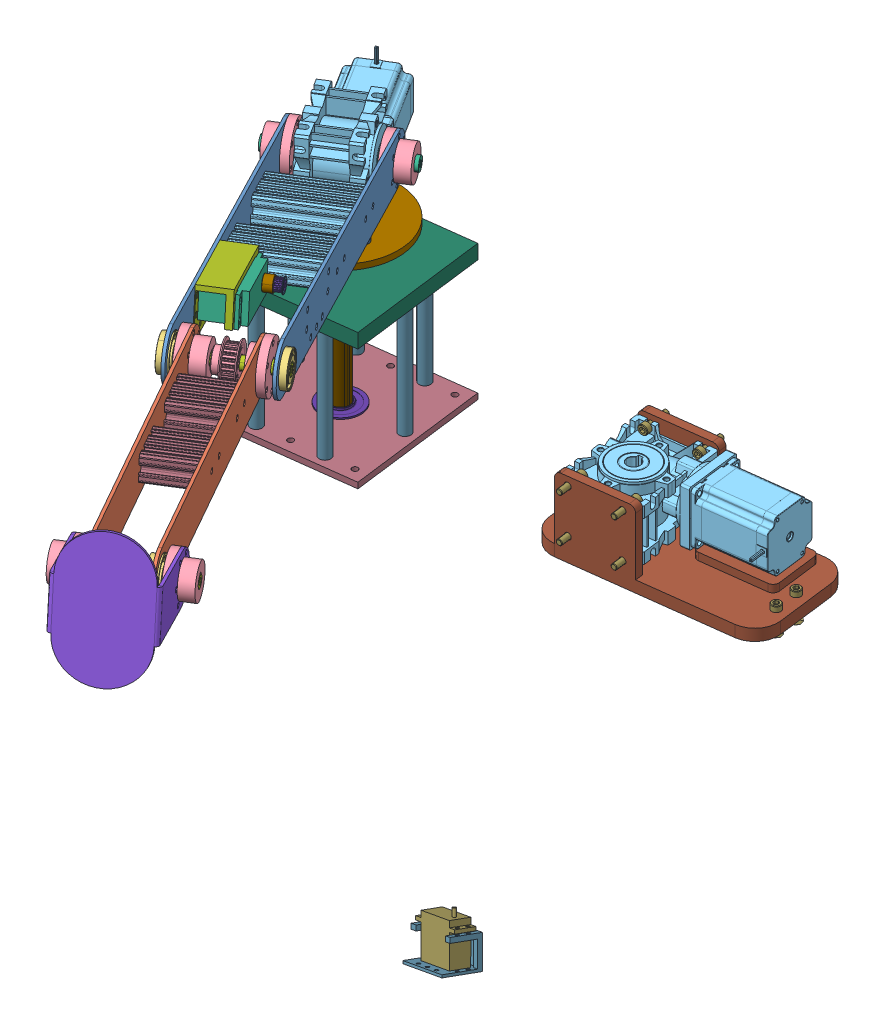
SolidWorks assembly Arm Assembly, configuration Default. Lengths in mm.
Overall size (689.03 483.25 867.03).
72 component instances, 32 part files, 136 mates.
Components (placement in the parent):
- Link 2-1: Link 2 [Default] at (-46.0857 347.5662 397.2138) x (0.521473 0.189246 0.832017) z (0.847329 0 -0.531069) size (457.2 50.8 3.17)
- Link 3-1: Link 3 [Default] at (228.0517 424.7546 698.466) x (0.527308 0.118805 0.841327) z (0.847329 0 -0.531069) size (406.4 50.8 3.17)
- Flanged Bearing-1: Flanged Bearing [Default] at (372.8529 441.7816 1027.9719) x (-0.531069 0 -0.847329) z (0.847329 0 -0.531069) size (38.1 38.1 12.7)
- Keyed hub-1: Keyed hub [Default] at (25.196 322.6251 358.2104) x (-0.50186 0.327073 -0.800725) z (-0.173699 -0.944999 -0.277139) size (50.8 25.4 50.8)
- Link 2-2: Link 2 [Default] at (29.3689 347.5662 349.9221) x (0.521473 0.189246 0.832017) z (0.847329 0 -0.531069) size (457.2 50.8 3.17)
- Link 3-2: Link 3 [Default] at (180.9848 424.7546 727.9655) x (0.527308 0.118805 0.841327) z (0.847329 0 -0.531069) size (406.4 50.8 3.17)
- Flanged Bearing-2: Flanged Bearing [Default] at (246.603 399.5345 690.4002) x (0.505623 0.305833 0.806729) z (0.847329 0 -0.531069) size (38.1 38.1 12.7)
- Flanged Bearing-3: Flanged Bearing [Default] at (417.1004 441.7816 1000.2394) x (0.490568 -0.383029 0.782708) z (-0.847329 0 0.531069) size (38.1 38.1 12.7)
- Keyed hub-2: Keyed hub [Default] at (175.8617 399.5345 734.7378) x (-0.425115 -0.599347 -0.678278) z (0.318295 -0.800489 0.507844) size (50.8 25.4 50.8)
- Keyed hub-3: Keyed hub [Default] at (-34.117 322.6251 395.3853) x (0.50186 -0.327073 0.800725) z (-0.173699 -0.944999 -0.277139) size (50.8 25.4 50.8)
- Keyed hub-4: Keyed hub [Default] at (239.0702 399.5345 695.1214) x (0.425115 0.599347 0.678278) z (0.318295 -0.800489 0.507844) size (50.8 25.4 50.8)
- Flanged Bearing-4: Flanged Bearing [Default] at (168.329 399.5345 739.459) x (-0.489048 0.389858 -0.780284) z (-0.847329 0 0.531069) size (38.1 38.1 12.7)
- Nema Stepper Motor-2: Nema Stepper Motor [Default] at (-44.1852 303.6559 313.4165) x (-0.531069 0 -0.847329) z (-0.847329 0 0.531069) size (171.01 100.01 63.01)
- Keyed Drive Shaft-1: Keyed Drive Shaft [Default] at (-114.1958 326.1952 444.2905) x (-0.50186 0.327073 -0.800725) z (0.847329 0 -0.531069) size (19.9 19.9 128.01)
- Keyed Shaft-1: Keyed Shaft [Default] at (155.1338 399.5345 747.7291) x (-0.425115 -0.599347 -0.678278) z (0.847329 0 -0.531069) size (12.7 12.5 104.14)
- Link 4-1: Link 4 [Default] at (433.2352 482.2587 1073.4043) x (0.847329 0 -0.531069) z (-0.10549 0.980073 -0.168311) size (90.37 102.6 133.86)
- Keyed hub-5: Keyed hub [Default] at (366.8892 441.7816 1031.7096) x (0.520486 0.198637 0.830444) z (0.10549 -0.980073 0.168311) size (50.8 25.4 50.8)
- Keyed hub-6: Keyed hub [Default] at (424.6331 441.7816 995.5182) x (-0.520486 -0.198637 -0.830444) z (0.10549 -0.980073 0.168311) size (50.8 25.4 50.8)
- Keyed Shaft-2: Keyed Shaft [Default] at (454.7641 441.7816 976.6334) x (0.520486 0.198637 0.830444) z (-0.847329 0 0.531069) size (12.7 12.5 104.14)
- Joint 2 Motor Plate-1: Joint 2 Motor Plate [Default] at (-4.244 255.2751 376.7854) x (0.215278 0 -0.976553) z (0.976553 0 0.215278) size (127 6.35 127)
- 4 mm M6 spacer-1: 4 mm M6 spacer [94669A162] at (1.753 263.6251 341.1619) x (-0.888418 0 -0.459036) z (0 -1 0) size (13 13 4)
- 4 mm M6 spacer-2: 4 mm M6 spacer [94669A162] at (30.4307 263.6251 386.9176) x (0.999963 0 0.008554) z (0 -1 0) size (13 13 4)
- 4 mm M6 spacer-3: 4 mm M6 spacer [94669A162] at (-38.9188 263.6251 366.6532) x (1 0 0) z (0 -1 0) size (13 13 4)
- 4 mm M6 spacer-4: 4 mm M6 spacer [94669A162] at (-10.2411 263.6251 412.409) x (1 0 0) z (0 -1 0) size (13 13 4)
- Motor Mount Joint 1 Assembly-1: Motor Mount Joint 1 Assembly [Default] at (255.7253 -1.2672 148.6448) x (0.992107 0 -0.125391) z (0.125391 0 0.992107) size (228.6 94.85 140.08)
  - Joint 1 Motor Holder Bracket-1: Joint 1 Motor Holder Bracket [Default] at (55.8829 79.1234 191.166) size (228.6 82.55 114.78)
  - Nema Stepper Motor-1: Nema Stepper Motor [Default] at (81.7887 128.4828 180.6968) x (1 0 0) z (0 1 0) size (171.01 100.01 63.01)
  - Flanged Bearing-1: Flanged Bearing [Default] at (6.9829 88.5722 199.666) x (0.99323 0 0.116162) z (0 -1 0) size (38.1 38.1 12.7)
  - socket head cap screw_am-7: socket head cap screw_am [B18.3.1M - 6 x 1.0 x 25 Hex SHCS -- 25NHX] at (-20.0631 152.4828 153.666) x (0 0 -1) z (0.990069 0.140585 0) size (31 10 10)
  - socket head cap screw_am-8: socket head cap screw_am [B18.3.1M - 6 x 1.0 x 25 Hex SHCS -- 25NHX] at (33.9369 152.4828 228.666) x (0 0 1) z (-1 0 0) size (31 10 10)
  - socket head cap screw_am-9: socket head cap screw_am [B18.3.1M - 6 x 1.0 x 25 Hex SHCS -- 25NHX] at (-20.0631 152.4828 228.666) x (0 0 1) z (0.381849 0.924225 0) size (31 10 10)
  - socket head cap screw_am-10: socket head cap screw_am [B18.3.1M - 6 x 1.0 x 25 Hex SHCS -- 25NHX] at (-20.0631 104.4828 153.666) x (0 0 -1) z (0.756248 0.654286 0) size (31 10 10)
  - socket head cap screw_am-11: socket head cap screw_am [B18.3.1M - 6 x 1.0 x 25 Hex SHCS -- 25NHX] at (33.9369 104.4828 150.5881) x (0 0 -1) z (0.923728 0.383049 0) size (31 10 10)
  - socket head cap screw_am-12: socket head cap screw_am [B18.3.1M - 6 x 1.0 x 25 Hex SHCS -- 25NHX] at (-45.7171 97.8234 212.366) x (0 -1 0) z (-0.546944 0 0.837169) size (31 10 10)
  - socket head cap screw_am-19: socket head cap screw_am [B18.3.1M - 6 x 1.0 x 25 Hex SHCS -- 25NHX] at (-45.7171 97.8234 186.966) x (0 -1 0) z (-0.546944 0 0.837169) size (31 10 10)
  - socket head cap screw_am-14: socket head cap screw_am [B18.3.1M - 6 x 1.0 x 25 Hex SHCS -- 25NHX] at (33.9369 152.4828 153.666) x (0 0 -1) z (0.923728 0.383049 0) size (31 10 10)
  - socket head cap screw_am-15: socket head cap screw_am [B18.3.1M - 6 x 1.0 x 25 Hex SHCS -- 25NHX] at (157.4829 97.8234 186.966) x (0 -1 0) z (-0.546944 0 0.837169) size (31 10 10)
  - socket head cap screw_am-16: socket head cap screw_am [B18.3.1M - 6 x 1.0 x 25 Hex SHCS -- 25NHX] at (-20.0631 104.4828 228.666) x (0 0 1) z (-1 0 0) size (31 10 10)
  - socket head cap screw_am-17: socket head cap screw_am [B18.3.1M - 6 x 1.0 x 25 Hex SHCS -- 25NHX] at (33.9369 104.4828 228.666) x (0 0 1) z (-1 0 0) size (31 10 10)
  - socket head cap screw_am-18: socket head cap screw_am [B18.3.1M - 6 x 1.0 x 25 Hex SHCS -- 25NHX] at (157.4829 97.8234 212.366) x (0 -1 0) z (-0.546944 0 0.837169) size (31 10 10)
- Joint 1 bottom plate-1: Joint 1 bottom plate [89155K113] at (-4.244 81.0311 376.7854) x (-0.125391 0 -0.992107) z (0.992107 0 -0.125391) size (152.4 6.35 152.4)
- Base post-1: Base post [8974K269] at (21.393 160.4061 309.54) x (-0.837169 0 -0.546944) z (0 -1 0) size (12.7 12.7 127)
- Base post-2: Base post [8974K269] at (-29.8811 160.4061 444.0308) x (-0.837169 0 -0.546944) z (0 -1 0) size (12.7 12.7 127)
- Base post-3: Base post [8974K269] at (37.3177 160.4061 435.5376) x (0.463623 0 0.886032) z (0 -1 0) size (12.7 12.7 127)
- Base post-4: Base post [8974K269] at (58.7548 160.4061 368.8231) x (-0.837169 0 -0.546944) z (0 -1 0) size (12.7 12.7 127)
- Base post-5: Base post [8974K269] at (-70.4278 160.4061 359.5483) x (-0.837169 0 -0.546944) z (0 -1 0) size (12.7 12.7 127)
- Base post-6: Base post [8974K269] at (-45.8058 160.4061 318.0332) x (-0.837169 0 -0.546944) z (0 -1 0) size (12.7 12.7 127)
- Base post-7: Base post [8974K269] at (-64.0579 160.4061 409.9473) x (-0.837169 0 -0.546944) z (0 -1 0) size (12.7 12.7 127)
- Joint 1 top plate-1: Joint 1 top plate [89155K143] at (-4.244 219.1436 376.7854) x (-0.125391 0 -0.992107) z (0.992107 0 -0.125391) size (152.4 15.88 152.4)
- Tapered-Roller Bearing-1: Tapered-Roller Bearing [5709K77] at (-4.244 223.5886 376.7854) x (1 0 0) z (0 -1 0) size (45.24 45.24 17.1)
- base Ball Bearing 0.75 in-1: base Ball Bearing 0.75 in [6384K367] at (-4.244 79.4436 376.7854) x (1 0 0) z (0 -1 0) size (44.45 44.45 14.27)
- keyed shaft 0.75 in bore 9 in-1: keyed shaft 0.75 in bore 9 in [Default] at (-4.244 155.2626 376.7854) x (0.215278 0 -0.976553) z (0 -1 0) size (19.05 18.75 228.6)
- 0.75 in shaft hub-1: 0.75 in shaft hub [Default] at (-4.244 248.9251 376.7854) x (-0.215278 0 0.976553) z (0 -1 0) size (63.5 63.5 19.49)
- Clamping Two-Piece Shaft Collar 0.75 in-1: Clamping Two-Piece Shaft Collar 0.75 in [6436K16] at (-4.244 240.9876 376.7854) x (0.996685 0 0.081358) z (0 1 0) size (38.06 38.1 12.77)
- T-slot Slider-1: T-slot Slider [5278N52] at (236.9979 67.7205 365.0672) x (-0.837169 0 -0.546944) z (0 1 0) size (10 9.8 4.82)
- T-slot Slider-2: T-slot Slider [5278N52] at (233.8129 65.4156 339.8677) x (-0.837169 0 -0.546944) z (0 1 0) size (10 9.8 4.82)
- T-slot Slider-3: T-slot Slider [5278N52] at (438.5941 68.7454 339.5877) x (-0.838988 0 -0.544149) z (0 1 0) size (10 9.8 4.82)
- T-slot Slider-4: T-slot Slider [5278N52] at (435.4091 66.889 314.3882) x (-0.837169 0 -0.546944) z (0 1 0) size (10 9.8 4.82)
- joint3pulley-1: joint3pulley [6495K752] at (208.3994 399.5345 714.3446) x (-0.496066 -0.357037 -0.791481) z (-0.847329 0 0.531069) size (38.1 38.1 22.23)
- 8020tframeforjoint3-1: 8020tframeforjoint3 [47065T653] at (20.3369 341.8525 478.9955) x (-0.100502 0.98193 -0.160353) z (0.847329 0 -0.531069) size (25.4 50.8 85.85)
- 8020tframeforjoint3-2: 8020tframeforjoint3 [47065T653] at (73.3185 361.0798 563.5284) x (-0.100502 0.98193 -0.160353) z (0.847329 0 -0.531069) size (25.4 50.8 85.85)
- 80 kg-1: 80 kg [Default] at (126.7022 373.3731 665.4861) x (-0.521473 -0.189246 -0.832017) z (0.100502 -0.98193 0.160353) size (82 48 30)
- servobracket_80kg-1: servobracket_80kg [Default] at (108.1358 376.7277 637.298) x (-0.521473 -0.189246 -0.832017) z (0.100502 -0.98193 0.160353) size (87.12 31.24 59.67)
- 3422-0004-0020 assembly.STEP-1: 3422-0004-0020 assembly.STEP [Default] at (106.5575 368.2135 573.9097) x (-0.472745 -0.455616 -0.754272) z (0.241963 -0.890177 0.386056) size (15 18 15.01)
  - 3422-0004-0020 core.STEP-1: 3422-0004-0020 core.STEP [Default] at (-35.1952 21.4358 6.7264) size (12.22 18 12.22)
  - 3422 series barrel.STEP-1: 3422 series barrel.STEP [Default] at (-35.1952 8.9358 6.7264) x (1 0 0) z (0 1 0) size (15 15.01 9)
  - 3422 series flange.STEP-1: 3422 series flange.STEP [Default] at (-35.1952 24.9358 6.7264) x (1 0 0) z (0 1 0) size (15 15 1)
  - 2806-0005-0005_91390A117.STEP-1: 2806-0005-0005_91390A117.STEP [Default] at (-35.1952 13.4358 11.638) x (-0.412538 -0.91094 0) z (0 0 1) size (5.01 5.01 5.01)
- 25 kg-1: 25 kg [Default] at (537.5356 49.5478 829.9464) x (0.939938 0.302082 0.158944) z (-0.225843 0.201201 0.953159) size (55 48 20)
- 8020tframeforjoint4-1: 8020tframeforjoint4 [47065T653] at (290.0659 408.5875 752.4523) x (-0.063094 0.992918 -0.100667) z (-0.847329 0 0.531069) size (25.4 50.8 52.32)
- 8020tframeforjoint4-2: 8020tframeforjoint4 [47065T653] at (336.9436 419.1492 827.2463) x (0.063094 -0.992918 0.100667) z (-0.847329 0 0.531069) size (25.4 50.8 52.32)
- 25kgservobracket2-3: 25kgservobracket2 [Default] at (940.3101 476.6609 1737.7737) x (-0.939938 -0.302082 -0.158944) z (-0.255952 0.931807 -0.25734) size (55.12 37.85 31.5)
Mates (geometry in assembly coordinates):
- Concentric3: concentric aligned: cylinder of Keyed hub-1 through (31.9217 322.6251 353.9951) axis (0.847329 0 -0.531069) radius 17.4625; cylinder of Link 2-2 through (31.9217 322.6251 353.9951) axis (0.847329 0 -0.531069) radius 17.4625
- Coincident2: coincident anti-aligned: plane of Keyed hub-1 through (31.9217 322.6251 353.9951) normal (0.847329 0 -0.531069); plane of Link 2-2 through (31.9217 322.6251 353.9951) normal (-0.847329 0 0.531069)
- Concentric4: concentric aligned: cylinder of Keyed hub-1 through (21.3415 329.5205 337.1142) axis (0.847329 0 -0.531069) radius 2.5527; cylinder of Link 2-2 through (24.0317 329.5205 335.4281) axis (0.847329 0 -0.531069) radius 2.5527
- Concentric5: concentric anti-aligned: cylinder of Link 2-1 through (-43.5329 322.6251 401.2868) axis (0.847329 0 -0.531069) radius 17.4625; cylinder of Keyed hub-3 through (-40.8427 322.6251 399.6006) axis (-0.847329 0 0.531069) radius 17.4625
- Coincident3: coincident anti-aligned: plane of Link 2-1 through (-40.8427 322.6251 399.6006) normal (0.847329 0 -0.531069); plane of Keyed hub-3 through (-40.8427 322.6251 399.6006) normal (-0.847329 0 0.531069)
- Concentric7: concentric anti-aligned: cylinder of Link 2-1 through (-38.7239 301.9241 402.9812) axis (0.847329 0 -0.531069) radius 2.5527; cylinder of Keyed hub-3 through (-38.7239 301.9241 402.9812) axis (-0.847329 0 0.531069) radius 2.5527
- Concentric8: concentric anti-aligned: cylinder of Keyed hub-1 through (25.196 322.6251 358.2104) axis (0.847329 0 -0.531069) radius 6.35; cylinder of Keyed hub-3 through (-34.117 322.6251 395.3853) axis (-0.847329 0 0.531069) radius 6.35
- Coincident5: coincident aligned: plane of Keyed hub-1 through (25.9927 322.1059 359.4816) normal (-0.50186 0.327073 -0.800725); plane of Keyed hub-3 through (-33.3203 322.1059 396.6564) normal (-0.50186 0.327073 -0.800725)
- Concentric9: concentric aligned: cylinder of Link 2-2 through (243.8481 399.5345 692.1268) axis (0.847329 0 -0.531069) radius 17.4625; cylinder of Flanged Bearing-2 through (251.9835 399.5345 687.0279) axis (0.847329 0 -0.531069) radius 17.4625
- Concentric10: concentric anti-aligned: cylinder of Link 2-1 through (168.3935 399.5345 739.4185) axis (0.847329 0 -0.531069) radius 17.4625; cylinder of Flanged Bearing-4 through (162.9484 399.5345 742.8313) axis (-0.847329 0 0.531069) radius 17.4625
- Concentric11: concentric anti-aligned: cylinder of Link 3-1 through (229.6543 399.5345 701.0229) axis (0.847329 0 -0.531069) radius 17.4625; cylinder of Keyed hub-4 through (232.3445 399.5345 699.3368) axis (-0.847329 0 0.531069) radius 17.4625
- Coincident8: coincident anti-aligned: plane of Link 3-1 through (232.3445 399.5345 699.3368) normal (0.847329 0 -0.531069); plane of Keyed hub-4 through (232.3445 399.5345 699.3368) normal (-0.847329 0 0.531069)
- Concentric12: concentric anti-aligned: cylinder of Link 3-1 through (231.0144 420.4672 697.2145) axis (0.847329 0 -0.531069) radius 2.5527; cylinder of Keyed hub-4 through (231.0144 420.4672 697.2145) axis (-0.847329 0 0.531069) radius 2.5527
- Concentric13: concentric aligned: cylinder of Link 3-2 through (182.5874 399.5345 730.5225) axis (0.847329 0 -0.531069) radius 17.4625; cylinder of Keyed hub-2 through (182.5874 399.5345 730.5225) axis (0.847329 0 -0.531069) radius 17.4625
- Coincident9: coincident anti-aligned: plane of Link 3-2 through (182.5874 399.5345 730.5225) normal (-0.847329 0 0.531069); plane of Keyed hub-2 through (182.5874 399.5345 730.5225) normal (0.847329 0 -0.531069)
- Concentric14: concentric aligned: cylinder of Link 3-2 through (183.9475 420.4672 726.714) axis (0.847329 0 -0.531069) radius 2.5527; cylinder of Keyed hub-2 through (181.2572 420.4672 728.4002) axis (0.847329 0 -0.531069) radius 2.5527
- Concentric15: concentric anti-aligned: cylinder of Keyed hub-2 through (175.8617 399.5345 734.7378) axis (0.847329 0 -0.531069) radius 6.35; cylinder of Keyed hub-4 through (239.0702 399.5345 695.1214) axis (-0.847329 0 0.531069) radius 6.35
- Coincident10: coincident aligned: plane of Keyed hub-2 through (175.1868 398.5831 733.661) normal (0.425115 0.599347 0.678278); plane of Keyed hub-4 through (238.3953 398.5831 694.0447) normal (0.425115 0.599347 0.678278)
- Concentric16: concentric aligned: cylinder of Flanged Bearing-2 through (251.9835 399.5345 687.0279) axis (0.847329 0 -0.531069) radius 6.35; cylinder of Keyed hub-2 through (175.8617 399.5345 734.7378) axis (0.847329 0 -0.531069) radius 6.35
- Concentric17: concentric aligned: cylinder of Flanged Bearing-1 through (378.2334 441.7816 1024.5996) axis (0.847329 0 -0.531069) radius 17.4625; cylinder of Link 3-2 through (370.098 441.7816 1029.6985) axis (0.847329 0 -0.531069) radius 17.4625
- Coincident13: coincident anti-aligned: plane of Flanged Bearing-1 through (370.098 459.2441 1029.6985) normal (0.847329 0 -0.531069); plane of Link 3-2 through (182.5874 399.5345 730.5225) normal (-0.847329 0 0.531069)
- Concentric18: concentric anti-aligned: cylinder of Link 3-1 through (417.1649 441.7816 1000.199) axis (0.847329 0 -0.531069) radius 17.4625; cylinder of Flanged Bearing-3 through (411.7198 441.7816 1003.6117) axis (-0.847329 0 0.531069) radius 17.4625
- Coincident14: coincident anti-aligned: plane of Link 3-1 through (232.3445 399.5345 699.3368) normal (0.847329 0 -0.531069); plane of Flanged Bearing-3 through (423.4073 457.9123 1004.1803) normal (-0.847329 0 0.531069)
- Concentric21: concentric anti-aligned: cylinder of Keyed hub-1 through (25.196 322.6251 358.2104) axis (0.847329 0 -0.531069) radius 6.35; cylinder of Keyed Drive Shaft-1 through (49.7685 322.6251 342.8094) axis (-0.847329 0 0.531069) radius 7
- Parallel1: parallel anti-aligned: plane of Keyed hub-1 through (25.9927 322.1059 359.4816) normal (-0.50186 0.327073 -0.800725); plane of Keyed Drive Shaft-1 through (-2.2852 326.816 380.2685) normal (0.50186 -0.327073 0.800725)
- Coincident18: coincident anti-aligned: plane of Keyed hub-3 through (-34.117 322.6251 395.3853) normal (0.847329 0 -0.531069); plane of Keyed Drive Shaft-1 through (-32.3521 328.5578 398.2011) normal (-0.847329 0 0.531069)
- Coincident19: coincident anti-aligned: plane of Keyed hub-1 through (25.196 322.6251 358.2104) normal (-0.847329 0 0.531069); plane of Keyed Drive Shaft-1 through (26.9609 328.5578 361.0263) normal (0.847329 0 -0.531069)
- Concentric22: concentric anti-aligned: cylinder of Keyed hub-2 through (175.8617 399.5345 734.7378) axis (0.847329 0 -0.531069) radius 6.35; cylinder of Keyed Shaft-1 through (251.9835 399.5345 687.0279) axis (-0.847329 0 0.531069) radius 6.35
- Coincident20: coincident aligned: plane of Keyed hub-2 through (175.1868 398.5831 733.661) normal (0.425115 0.599347 0.678278); plane of Keyed Shaft-1 through (249.7968 402.3852 683.539) normal (0.425115 0.599347 0.678278)
- Coincident22: coincident anti-aligned: plane of Link 2-1 through (-40.8427 322.6251 399.6006) normal (0.847329 0 -0.531069); plane of Flanged Bearing-4 through (167.4683 383.4537 731.9639) normal (-0.847329 0 0.531069)
- Distance1: distance = 2.54 mm anti-aligned: plane of Flanged Bearing-4 through (171.3272 388.9387 732.2858) normal (0.847329 0 -0.531069); plane of Keyed hub-2 through (175.8617 399.5345 734.7378) normal (-0.847329 0 0.531069)
- Coincident24: coincident anti-aligned: plane of Link 2-2 through (31.9217 322.6251 353.9951) normal (-0.847329 0 0.531069); plane of Flanged Bearing-2 through (246.6844 382.9087 696.6521) normal (0.847329 0 -0.531069)
- Distance2: distance = 2.54 mm anti-aligned: plane of Keyed hub-4 through (239.0702 399.5345 695.1214) normal (0.847329 0 -0.531069); plane of Flanged Bearing-2 through (243.0912 388.5796 696.7542) normal (-0.847329 0 0.531069)
- Coincident26: coincident aligned: plane of Flanged Bearing-2 through (253.0149 393.4888 688.6735) normal (0.847329 0 -0.531069); plane of Keyed Shaft-1 through (251.9835 399.5345 687.0279) normal (0.847329 0 -0.531069)
- Concentric23: concentric anti-aligned: cylinder of Link 4-1 through (434.0491 441.7816 989.6167) axis (-0.847329 0 0.531069) radius 17.4625; cylinder of Keyed hub-6 through (431.3588 441.7816 991.3029) axis (0.847329 0 -0.531069) radius 17.4625
- Concentric24: concentric anti-aligned: cylinder of Link 4-1 through (423.9463 457.5815 979.4762) axis (-0.847329 0 0.531069) radius 2.5527; cylinder of Keyed hub-6 through (423.9463 457.5815 979.4762) axis (0.847329 0 -0.531069) radius 2.5527
- Coincident27: coincident anti-aligned: plane of Link 4-1 through (490.1801 490.4056 1085.1531) normal (-0.847329 0 0.531069); plane of Keyed hub-6 through (431.3588 441.7816 991.3029) normal (0.847329 0 -0.531069)
- Concentric25: concentric anti-aligned: cylinder of Link 4-1 through (357.4733 441.7816 1037.6111) axis (0.847329 0 -0.531069) radius 17.4625; cylinder of Keyed hub-5 through (360.1635 441.7816 1035.925) axis (-0.847329 0 0.531069) radius 17.4625
- Concentric26: concentric anti-aligned: cylinder of Link 4-1 through (352.7511 457.5815 1024.0983) axis (0.847329 0 -0.531069) radius 2.5527; cylinder of Keyed hub-5 through (352.7511 457.5815 1024.0983) axis (-0.847329 0 0.531069) radius 2.5527
- Concentric27: concentric anti-aligned: cylinder of Keyed hub-5 through (366.8892 441.7816 1031.7096) axis (-0.847329 0 0.531069) radius 6.35; cylinder of Keyed Shaft-2 through (357.9145 441.7816 1037.3346) axis (0.847329 0 -0.531069) radius 6.35
- Coincident31: coincident aligned: plane of Keyed hub-5 through (366.0629 441.4662 1030.3913) normal (0.520486 0.198637 0.830444); plane of Keyed Shaft-2 through (356.5871 446.1214 1035.2168) normal (0.520486 0.198637 0.830444)
- Coincident32: coincident aligned: plane of Keyed hub-6 through (446.1553 441.7816 982.0291) normal (0.847329 0 -0.531069); plane of Keyed Shaft-2 through (446.1553 441.7816 982.0291) normal (0.847329 0 -0.531069)
- Coincident34: coincident anti-aligned: plane of Link 4-1 through (418.9848 490.4056 1129.7752) normal (0.847329 0 -0.531069); plane of Keyed hub-5 through (360.1635 441.7816 1035.925) normal (-0.847329 0 0.531069)
- Coincident36: coincident aligned: plane of Keyed hub-6 through (425.4594 442.0969 996.8366) normal (-0.520486 -0.198637 -0.830444); plane of Keyed Shaft-2 through (358.2397 446.7521 1037.8535) normal (-0.520486 -0.198637 -0.830444)
- Concentric28: concentric anti-aligned: cone of Flanged Bearing-3 through (421.9135 441.7816 997.2228) axis (-0.847329 0 0.531069); cylinder of Keyed Shaft-2 through (357.9145 441.7816 1037.3346) axis (0.847329 0 -0.531069) radius 6.35
- Distance3: distance = 2.54 mm anti-aligned: plane of Flanged Bearing-3 through (424.8214 452.4103 1000.6015) normal (0.847329 0 -0.531069); plane of Keyed hub-6 through (424.6331 441.7816 995.5182) normal (-0.847329 0 0.531069)
- Coincident38: coincident anti-aligned: plane of Top base plate-1 through (74.0847 244.0001 261.2257) normal (0 -1 0); plane of arm base spacer small part-1 through (130.8381 244.0001 364.6329) normal (0 1 0)
- Coincident40: coincident anti-aligned: plane of Top base plate-1 through (74.0847 244.0001 261.2257) normal (0 -1 0); plane of arm base spacer large part-1 through (32.1724 244.0001 346.1862) normal (0 1 0)
- Coincident45: coincident anti-aligned: plane of Bearing other part-1 through (32.1724 247.1751 346.1862) normal (0 -1 0); plane of Top base plate-1 through (74.0847 247.1751 261.2257) normal (0 1 0)
- Concentric32: concentric aligned: cylinder of Bearing other part-1 through (32.1724 257.1751 346.1862) axis (0 -1 0) radius 70; circle of arm base spacer large part-1
- Coincident57: coincident aligned: plane of Top base plate-1 through (-6.0476 247.1751 446.2586) normal (0.059501 0 0.998228); plane of arm base spacer large part-1 through (84.7912 244.0001 440.844) normal (0.059501 0 0.998228)
- Coincident58: coincident aligned: plane of Top base plate-1 through (-75.7951 247.1751 376.9496) normal (-0.998228 0 0.059501); plane of arm base spacer large part-1 through (-75.8042 244.0001 376.7975) normal (-0.998228 0 0.059501)
- Concentric37: concentric aligned: cylinder of Top base plate-1 through (130.8381 247.1751 364.6329) axis (0 -1 0) radius 15; cylinder of arm base spacer small part-1 through (130.8381 244.0001 364.6329) axis (0 -1 0) radius 15
- Coincident59: coincident aligned: plane of Top base plate-1 through (145.8116 247.1751 363.7404) normal (0.998228 0 -0.059501); plane of arm base spacer small part-1 through (145.8116 244.0001 363.7404) normal (0.998228 0 -0.059501)
- Parallel2: parallel aligned: plane of Nema Stepper Motor-3 through (350.3499 203.0272 320.7095) normal (0 1 0); plane of Top base plate-1 through (74.0847 247.1751 261.2257) normal (0 1 0)
- Parallel3: parallel anti-aligned: plane of Nema Stepper Motor-3 through (312.2058 175.0272 353.0364) normal (-0.998228 0 0.059501); plane of arm base spacer small part-1 through (145.8116 244.0001 363.7404) normal (0.998228 0 -0.059501)
- Coincident61: coincident anti-aligned: plane of Nema Stepper Motor-2 through (-1.9757 265.6251 328.0385) normal (0 -1 0); plane of 4 mm M6 spacer-1 through (1.753 265.6251 341.1619) normal (0 1 0)
- Concentric43: concentric aligned: cylinder of Keyed hub-1 through (31.9217 322.6251 353.9951) axis (0.847329 0 -0.531069) radius 17.4625; cylinder of Nema Stepper Motor-2 through (-83.0293 322.6251 426.0414) axis (0.847329 0 -0.531069) radius 7
- Coincident65: coincident anti-aligned: plane of Nema Stepper Motor-2 through (22.2327 322.6251 360.0729) normal (0.847329 0 -0.531069); plane of Keyed Drive Shaft-1 through (22.2304 322.6251 360.0692) normal (-0.847329 0 0.531069)
- Concentric44: concentric aligned: cylinder of Joint 1 bottom plate-1 through (58.7548 83.9521 368.8231) axis (0 1 0) radius 1.905; cylinder of Base post-4 through (58.7548 84.2061 368.8231) axis (0 1 0) radius 6.35
- Concentric45: concentric aligned: cylinder of Joint 1 bottom plate-1 through (37.3177 83.9521 435.5376) axis (0 1 0) radius 1.905; cylinder of Base post-3 through (37.3177 84.2061 435.5376) axis (0 1 0) radius 6.35
- Concentric46: concentric aligned: cylinder of Joint 1 bottom plate-1 through (-29.8811 83.9521 444.0308) axis (0 1 0) radius 1.905; cylinder of Base post-2 through (-29.8811 84.2061 444.0308) axis (0 1 0) radius 6.35
- Concentric47: concentric aligned: cylinder of Joint 1 bottom plate-1 through (21.393 83.9521 309.54) axis (0 1 0) radius 1.905; cylinder of Base post-1 through (21.393 84.2061 309.54) axis (0 1 0) radius 6.35
- Concentric48: concentric aligned: cylinder of Joint 1 bottom plate-1 through (-45.8058 83.9521 318.0332) axis (0 1 0) radius 1.905; cylinder of Base post-6 through (-45.8058 84.2061 318.0332) axis (0 1 0) radius 6.35
- Concentric49: concentric aligned: cylinder of Joint 1 bottom plate-1 through (-64.0579 83.9521 409.9473) axis (0 1 0) radius 1.905; cylinder of Base post-7 through (-64.0579 84.2061 409.9473) axis (0 1 0) radius 6.35
- Concentric50: concentric aligned: cylinder of Joint 1 bottom plate-1 through (-70.4278 83.9521 359.5483) axis (0 1 0) radius 1.905; cylinder of Base post-5 through (-70.4278 84.2061 359.5483) axis (0 1 0) radius 6.35
- Coincident66: coincident anti-aligned: plane of Joint 1 bottom plate-1 through (80.9094 84.2061 442.8292) normal (0 1 0); plane of Base post-4 through (58.7548 84.2061 368.8231) normal (0 -1 0)
- Coincident67: coincident anti-aligned: plane of Joint 1 bottom plate-1 through (80.9094 84.2061 442.8292) normal (0 1 0); plane of Base post-3 through (37.3177 84.2061 435.5376) normal (0 -1 0)
- Coincident68: coincident anti-aligned: plane of Joint 1 bottom plate-1 through (80.9094 84.2061 442.8292) normal (0 1 0); plane of Base post-2 through (-29.8811 84.2061 444.0308) normal (0 -1 0)
- Coincident69: coincident anti-aligned: plane of Joint 1 bottom plate-1 through (80.9094 84.2061 442.8292) normal (0 1 0); plane of Base post-7 through (-64.0579 84.2061 409.9473) normal (0 -1 0)
- Coincident70: coincident anti-aligned: plane of Joint 1 bottom plate-1 through (80.9094 84.2061 442.8292) normal (0 1 0); plane of Base post-1 through (21.393 84.2061 309.54) normal (0 -1 0)
- Coincident71: coincident anti-aligned: plane of Joint 1 bottom plate-1 through (80.9094 84.2061 442.8292) normal (0 1 0); plane of Base post-6 through (-45.8058 84.2061 318.0332) normal (0 -1 0)
- Coincident72: coincident anti-aligned: plane of Joint 1 bottom plate-1 through (80.9094 84.2061 442.8292) normal (0 1 0); plane of Base post-5 through (-70.4278 84.2061 359.5483) normal (0 -1 0)
- Coincident73: coincident aligned: plane of Joint 1 bottom plate-1 through (71.3545 81.0311 367.2306) normal (0.992107 0 -0.125391); plane of Joint 1 top plate-1 through (71.3545 219.1436 367.2306) normal (0.992107 0 -0.125391)
- Coincident74: coincident aligned: plane of Joint 1 bottom plate-1 through (80.9094 77.8561 442.8292) normal (0.125391 0 0.992107); plane of Joint 1 top plate-1 through (80.9094 211.2061 442.8292) normal (0.125391 0 0.992107)
- Coincident75: coincident anti-aligned: plane of Base post-3 through (37.3177 211.2061 435.5376) normal (0 1 0); plane of Joint 1 top plate-1 through (61.7997 211.2061 291.632) normal (0 -1 0)
- Parallel5: parallel aligned: plane of Motor Mount Joint 1 Assembly-1/Joint 1 Motor Holder Bracket-1 through (228.936 90.5561 402.5641) normal (0.125391 0 0.992107); plane of Joint 1 bottom plate-1 through (80.9094 77.8561 442.8292) normal (0.125391 0 0.992107)
- Coincident79: coincident anti-aligned: plane of Joint 1 top plate-1 through (-4.244 217.5561 376.7854) normal (0 1 0); plane of Tapered-Roller Bearing-1 through (-4.244 217.5561 399.4073) normal (0 -1 0)
- Concentric51: concentric anti-aligned: cylinder of Joint 1 top plate-1 through (-4.244 217.5561 376.7854) axis (0 1 0) radius 22.6219; cylinder of Tapered-Roller Bearing-1 through (-4.244 223.5886 376.7854) axis (0 -1 0) radius 22.6219
- Coincident80: coincident anti-aligned: plane of Nema Stepper Motor-2 through (-1.9757 265.6251 328.0385) normal (0 -1 0); plane of 4 mm M6 spacer-2 through (30.4307 265.6251 386.9176) normal (0 1 0)
- Coincident81: coincident anti-aligned: plane of Nema Stepper Motor-2 through (-1.9757 265.6251 328.0385) normal (0 -1 0); plane of 4 mm M6 spacer-4 through (-10.2411 265.6251 412.409) normal (0 1 0)
- Concentric52: concentric anti-aligned: cylinder of Joint 1 bottom plate-1 through (-4.244 77.8561 376.7854) axis (0 1 0) radius 20.6375; cylinder of base Ball Bearing 0.75 in-1 through (-4.244 73.0936 376.7854) axis (0 -1 0) radius 20.6375
- Coincident82: coincident anti-aligned: plane of Joint 1 bottom plate-1 through (80.9094 84.2061 442.8292) normal (0 1 0); plane of base Ball Bearing 0.75 in-1 through (-4.244 84.2061 395.7927) normal (0 -1 0)
- Concentric53: concentric anti-aligned: cylinder of base Ball Bearing 0.75 in-1 through (-4.244 73.0936 376.7854) axis (0 -1 0) radius 9.525; cylinder of keyed shaft 0.75 in bore-1 through (-4.244 -126.3486 376.7854) axis (0 1 0) radius 9.525
- Concentric54: concentric anti-aligned: cylinder of base Ball Bearing 0.75 in-1 through (-4.244 73.0936 376.7854) axis (0 -1 0) radius 9.525; cylinder of keyed shaft 0.75 in bore 9 in-1 through (-4.244 40.9626 376.7854) axis (0 1 0) radius 9.525
- Coincident83: coincident aligned: plane of Motor Mount Joint 1 Assembly-1/Joint 1 Motor Holder Bracket-1 through (335.1377 77.8561 331.2948) normal (0 -1 0); plane of Joint 1 bottom plate-1 through (61.7997 77.8561 291.632) normal (0 -1 0)
- Concentric55: concentric aligned: cylinder of Joint 2 Motor Plate-1 through (-4.244 255.2751 376.7854) axis (0 1 0) radius 20.6375; circle of 0.75 in shaft hub-1
- Concentric56: concentric anti-aligned: cylinder of Joint 2 Motor Plate-1 through (-25.6499 255.2751 390.4583) axis (0 1 0) radius 3.175; circle of 0.75 in shaft hub-1
- Concentric57: concentric aligned: cylinder of keyed shaft 0.75 in bore 9 in-1 through (-4.244 40.9626 376.7854) axis (0 1 0) radius 9.525; cylinder of 0.75 in shaft hub-1 through (-4.244 247.3376 376.7854) axis (0 1 0) radius 9.525
- Parallel6: parallel aligned: plane of keyed shaft 0.75 in bore 9 in-1 through (2.212 40.9626 380.6536) normal (0.215278 0 -0.976553); plane of 0.75 in shaft hub-1 through (6.8704 248.9251 381.674) normal (0.215278 0 -0.976553)
- Coincident90: coincident anti-aligned: plane of Joint 2 Motor Plate-1 through (-4.244 255.2751 376.7854) normal (0 -1 0); plane of 0.75 in shaft hub-1 through (-4.244 255.2751 376.7854) normal (0 1 0)
- Concentric60: concentric anti-aligned: cylinder of keyed shaft 0.75 in bore 9 in-1 through (-4.244 40.9626 376.7854) axis (0 1 0) radius 9.525; cylinder of Clamping Two-Piece Shaft Collar 0.75 in-1 through (-4.244 247.3376 376.7854) axis (0 -1 0) radius 9.525
- Distance7: distance = 1.5875 mm anti-aligned: plane of Tapered-Roller Bearing-1 through (-4.244 233.0501 386.3104) normal (0 1 0); plane of Clamping Two-Piece Shaft Collar 0.75 in-1 through (-4.244 234.6376 376.7854) normal (0 -1 0)
- Distance8: distance = 1.5875 mm anti-aligned: plane of Clamping Two-Piece Shaft Collar 0.75 in-1 through (-4.244 247.3376 376.7854) normal (0 1 0); plane of 0.75 in shaft hub-1 through (-4.244 248.9251 376.7854) normal (0 -1 0)
- Distance9: distance = 1.5875 mm aligned: plane of keyed shaft 0.75 in bore 9 in-1 through (-4.244 269.5626 376.7854) normal (0 1 0); plane of 0.75 in shaft hub-1 through (-4.244 267.9751 376.7854) normal (0 1 0)
- Coincident95: coincident anti-aligned: plane of Nema Stepper Motor-2 through (-1.9757 265.6251 328.0385) normal (0 -1 0); plane of 4 mm M6 spacer-3 through (-38.9188 265.6251 366.6532) normal (0 1 0)
- Coincident96: coincident anti-aligned: plane of Joint 2 Motor Plate-1 through (-4.244 261.6251 376.7854) normal (0 1 0); plane of 4 mm M6 spacer-3 through (-38.9188 261.6251 366.6532) normal (0 -1 0)
- Concentric62: concentric anti-aligned: cylinder of Joint 2 Motor Plate-1 through (1.753 255.2751 341.1619) axis (0 1 0) radius 3.25; cylinder of 4 mm M6 spacer-1 through (1.753 265.6251 341.1619) axis (0 -1 0) radius 3.15
- Concentric63: concentric anti-aligned: cylinder of Joint 2 Motor Plate-1 through (30.4307 255.2751 386.9176) axis (0 1 0) radius 3.25; cylinder of 4 mm M6 spacer-2 through (30.4307 265.6251 386.9176) axis (0 -1 0) radius 3.15
- Tangent1: tangent anti-aligned: plane of Nema Stepper Motor-2 through (1.5702 288.3265 344.994) normal (-0.531069 0 -0.847329); cylinder of 4 mm M6 spacer-1 through (1.753 265.6251 341.1619) axis (0 -1 0) radius 3.15
- Tangent2: tangent anti-aligned: plane of Nema Stepper Motor-2 through (30.2479 288.3265 390.7498) normal (-0.531069 0 -0.847329); cylinder of 4 mm M6 spacer-2 through (30.4307 265.6251 386.9176) axis (0 -1 0) radius 3.15
- Tangent3: tangent anti-aligned: plane of Nema Stepper Motor-2 through (-35.7123 288.3265 368.3611) normal (-0.531069 0 -0.847329); cylinder of 4 mm M6 spacer-3 through (-38.9188 265.6251 366.6532) axis (0 -1 0) radius 3.15
- Concentric67: concentric anti-aligned: cylinder of Joint 2 Motor Plate-1 through (-10.2411 255.2751 412.409) axis (0 1 0) radius 3.25; cylinder of 4 mm M6 spacer-4 through (-10.2411 265.6251 412.409) axis (0 -1 0) radius 3.15
- Tangent5: tangent anti-aligned: plane of Nema Stepper Motor-2 through (-7.0345 288.3265 414.1168) normal (-0.531069 0 -0.847329); cylinder of 4 mm M6 spacer-4 through (-10.2411 265.6251 412.409) axis (0 -1 0) radius 3.15
- Concentric68: concentric anti-aligned: cylinder of Joint 2 Motor Plate-1 through (-38.9188 255.2751 366.6532) axis (0 1 0) radius 3.25; cylinder of 4 mm M6 spacer-3 through (-38.9188 265.6251 366.6532) axis (0 -1 0) radius 3.15
- Distance11: distance = 3.81 mm: point of 4 mm M6 spacer-1; plane of Nema Stepper Motor-2 through (19.2671 322.6251 361.9317) normal (0.847329 0 -0.531069)
- Concentric69: concentric aligned: cylinder of Motor Mount Joint 1 Assembly-1/socket head cap screw_am-18 through (438.5941 128.3061 339.5877) axis (0 1 0) radius 3; circle of T-slot Slider-3
- Concentric70: concentric aligned: cylinder of Motor Mount Joint 1 Assembly-1/socket head cap screw_am-15 through (435.4091 128.3061 314.3882) axis (0 1 0) radius 3; circle of T-slot Slider-4
- Concentric71: concentric aligned: cylinder of Motor Mount Joint 1 Assembly-1/socket head cap screw_am-12 through (236.9979 128.3061 365.0672) axis (0 1 0) radius 3; circle of T-slot Slider-1
- Concentric72: concentric aligned: cylinder of Motor Mount Joint 1 Assembly-1/socket head cap screw_am-19 through (233.8129 128.3061 339.8677) axis (0 1 0) radius 3; circle of T-slot Slider-2
- Concentric74: concentric anti-aligned: cylinder of Link 2-2 through (91.526 344.2559 449.0946) axis (0.847329 0 -0.531069) radius 2.794; cylinder of 8020tframeforjoint3-1 through (91.526 344.2559 449.0946) axis (-0.847329 0 0.531069) radius 2.6035
- Concentric75: concentric anti-aligned: cylinder of Link 2-2 through (78.2806 339.4491 427.9614) axis (0.847329 0 -0.531069) radius 2.794; cylinder of 8020tframeforjoint3-1 through (78.2806 339.4491 427.9614) axis (-0.847329 0 0.531069) radius 2.6035
- Coincident98: coincident anti-aligned: plane of Link 2-2 through (31.9217 322.6251 353.9951) normal (-0.847329 0 0.531069); plane of 8020tframeforjoint3-1 through (71.7265 341.338 417.5043) normal (0.847329 0 -0.531069)
- Concentric76: concentric anti-aligned: cylinder of Link 2-2 through (144.5076 363.4833 533.6276) axis (0.847329 0 -0.531069) radius 2.794; cylinder of 8020tframeforjoint3-2 through (144.5076 363.4833 533.6276) axis (-0.847329 0 0.531069) radius 2.6035
- Concentric77: concentric anti-aligned: cylinder of Link 2-2 through (131.2622 358.6764 512.4943) axis (0.847329 0 -0.531069) radius 2.794; cylinder of 8020tframeforjoint3-2 through (131.2622 358.6764 512.4943) axis (-0.847329 0 0.531069) radius 2.6035
- Coincident99: coincident anti-aligned: plane of Link 2-2 through (31.9217 322.6251 353.9951) normal (-0.847329 0 0.531069); plane of 8020tframeforjoint3-2 through (124.7081 360.5654 502.0372) normal (0.847329 0 -0.531069)
- Coincident100: coincident anti-aligned: plane of 80 kg-1 through (126.7022 373.3731 665.4861) normal (-0.847329 0 0.531069); plane of servobracket_80kg-1 through (108.7815 376.7277 636.8934) normal (0.847329 0 -0.531069)
- Concentric78: concentric aligned: cylinder of 80 kg-1 through (87.8373 383.2013 603.4766) axis (0.847329 0 -0.531069) radius 3; cylinder of servobracket_80kg-1 through (87.1917 383.2013 603.8813) axis (0.847329 0 -0.531069) radius 3
- Concentric79: concentric aligned: cylinder of 80 kg-1 through (128.6563 380.7019 668.6039) axis (0.847329 0 -0.531069) radius 3; cylinder of servobracket_80kg-1 through (128.0107 380.7019 669.0086) axis (0.847329 0 -0.531069) radius 3
- Concentric80: concentric aligned: cylinder of 80 kg-1 through (138.7499 378.2613 594.3246) axis (-0.847329 0 0.531069) radius 2; cylinder of 3422-0004-0020 assembly.STEP-1/3422-0004-0020 core.STEP-1 through (158.0079 378.2613 582.2545) axis (-0.847329 0 0.531069) radius 2
- Coincident101: coincident anti-aligned: plane of 80 kg-1 through (161.019 373.3731 643.9778) normal (0.847329 0 -0.531069); plane of 3422-0004-0020 assembly.STEP-1/3422 series barrel.STEP-1 through (132.3949 378.2613 598.3076) normal (-0.847329 0 0.531069)
- Coincident102: coincident anti-aligned: plane of Link 2-1 through (-40.8427 322.6251 399.6006) normal (0.847329 0 -0.531069); plane of servobracket_80kg-1 through (108.1358 376.7277 637.298) normal (-0.847329 0 0.531069)
- Concentric83: concentric aligned: cylinder of Link 2-1 through (107.1851 359.7318 641.7597) axis (0.847329 0 -0.531069) radius 3.048; circle of servobracket_80kg-1
- Concentric85: concentric aligned: cylinder of Link 2-1 through (96.5888 355.8863 624.8531) axis (0.847329 0 -0.531069) radius 3.048; cylinder of servobracket_80kg-1 through (99.2791 355.8863 623.167) axis (0.847329 0 -0.531069) radius 3
- Concentric86: concentric aligned: cylinder of Link 2-1 through (117.7815 363.5773 658.6663) axis (0.847329 0 -0.531069) radius 3.048; cylinder of servobracket_80kg-1 through (120.4717 363.5773 656.9801) axis (0.847329 0 -0.531069) radius 3
- Concentric91: concentric aligned: cylinder of Keyed Shaft-1 through (251.9835 399.5345 687.0279) axis (-0.847329 0 0.531069) radius 6.35; cylinder of joint3pulley-1 through (198.9835 399.5345 720.2461) axis (-0.847329 0 0.531069) radius 6.35
- Parallel10: parallel aligned: cylinder of joint3pulley-1 through (198.9835 399.5345 720.2461) axis (-0.847329 0 0.531069) radius 19.05; cylinder of 3422-0004-0020 assembly.STEP-1/3422 series flange.STEP-1 through (146.7995 378.2613 589.2795) axis (-0.847329 0 0.531069) radius 7.5
- Coincident111: coincident anti-aligned: plane of Link 3-1 through (229.6543 399.5345 701.0229) normal (-0.847329 0 0.531069); plane of 8020tframeforjoint4-1 through (269.8351 408.5875 765.1321) normal (0.847329 0 -0.531069)
- Concentric96: concentric aligned: cylinder of Link 3-1 through (263.1383 407.0786 754.4472) axis (0.847329 0 -0.531069) radius 2.794; cylinder of 8020tframeforjoint4-1 through (218.8027 407.0786 782.2349) axis (0.847329 0 -0.531069) radius 2.6035
- Concentric97: concentric aligned: cylinder of Link 3-1 through (276.5319 410.0963 775.817) axis (0.847329 0 -0.531069) radius 2.794; cylinder of 8020tframeforjoint4-1 through (232.1963 410.0963 803.6046) axis (0.847329 0 -0.531069) radius 2.6035
- Coincident115: coincident anti-aligned: plane of Link 3-1 through (229.6543 399.5345 701.0229) normal (-0.847329 0 0.531069); plane of 8020tframeforjoint4-2 through (316.7128 419.1492 839.9261) normal (0.847329 0 -0.531069)
- Concentric99: concentric aligned: cylinder of Link 3-1 through (323.4096 420.658 850.611) axis (0.847329 0 -0.531069) radius 2.794; cylinder of 8020tframeforjoint4-2 through (279.074 420.658 878.3986) axis (0.847329 0 -0.531069) radius 2.6035
- Concentric101: concentric aligned: cylinder of Link 3-1 through (310.016 417.6404 829.2412) axis (0.847329 0 -0.531069) radius 2.794; cylinder of 8020tframeforjoint4-2 through (265.6804 417.6404 857.0289) axis (0.847329 0 -0.531069) radius 2.6035
- Coincident140: coincident anti-aligned: plane of 25 kg-1 through (537.5356 49.5478 829.9464) normal (0.255952 -0.931807 0.25734); plane of 25kgservobracket2-3 through (955.9938 419.5637 1753.5425) normal (-0.255952 0.931807 -0.25734)
- Concentric104: concentric aligned: cylinder of 25 kg-1 through (535.1401 47.409 824.5845) axis (-0.255952 0.931807 -0.25734) radius 1.875; cylinder of 25kgservobracket2-3 through (535.7902 45.0422 825.2382) axis (-0.255952 0.931807 -0.25734) radius 1.875
- Concentric105: concentric aligned: cylinder of 25 kg-1 through (579.7871 61.7579 832.1344) axis (-0.255952 0.931807 -0.25734) radius 1.875; cylinder of 25kgservobracket2-3 through (580.4373 59.3911 832.7881) axis (-0.255952 0.931807 -0.25734) radius 1.875
